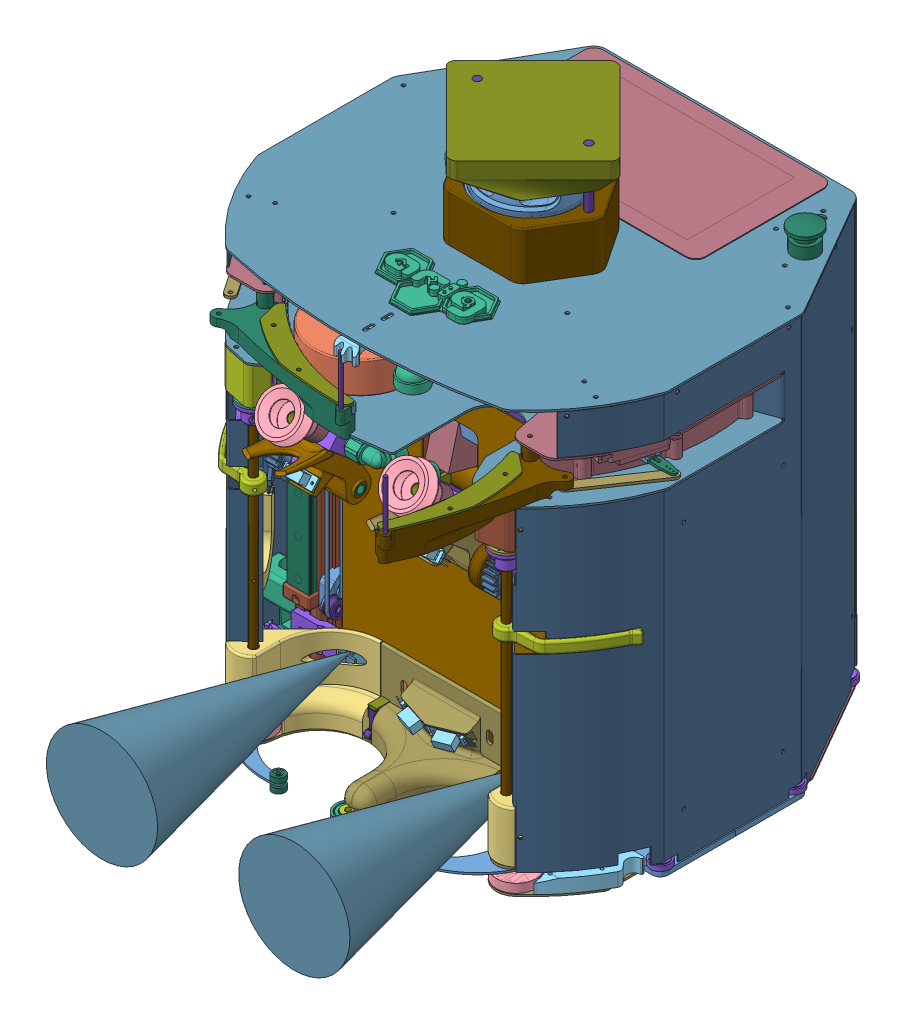
SolidWorks assembly 2019_Gros_robot, configuration Défaut. Lengths in mm. (continued)
Components (placement in the parent): (continued)
- 20181005-1508-1: 20181005-1508 [Défaut] at (-50 277.5 -86.6025) x (0 0 1) z (-1 0 0) size (212.1 303.52 220.42)
  - 20181005-1449-1: 20181005-1449 [Défaut] at (-40 0 0) size (80 80 0) (hidden)
  - 20181005-1520-1: 20181005-1520 [Défaut] at (40 -35 0) x (-0.992278 0.124035 0) z (0 0 -1) size (48.31 18.76 50.57)
  - 20181005-1525-1: 20181005-1525 [Défaut] at (30 -50 0) x (-0.986394 0.164399 0) z (0 0 -1) size (38.41 16.66 50.83)
  - 20181005-1532-1: 20181005-1532 [Défaut] at origin size (84 50 84)
  - Rotule Rose-1: Rotule Rose [aligné] at (33.0169 -69.1373 7) x (0.894203 -0.447662 0) z (-0.447662 -0.894203 0) size (18 6.89 7.5)
    - Rotule Rose piece01-1: Rotule Rose piece01 [Défaut] at origin size (5.4 6 5.4)
    - Rotule Rose piece02-1: Rotule Rose piece02 [Défaut] x (-1 0 0) z (0 0 -1) size (18 5.77 7.5)
  - Rotule noire-2: Rotule noire [Aligné] at (3.5082 -54.3644 7) x (0.894203 -0.447662 0) z (-0.447662 -0.894203 0) size (19 15.5 6.5)
    - Rotule noire piece01-1: Rotule noire piece01 [Défaut] at origin size (6.35 14.5 5.5)
    - Rotule noire piece02-1: Rotule noire piece02 [Défaut] at origin size (19 6 6.5)
  - Rondelle-M3-1: Rondelle-M3 [Défaut] at (40 -35 25) x (0.373687 0.927555 0) z (0 0 1) size (8 8 0.8)
  - EcrouFrein_H-M3-1: EcrouFrein_H-M3 [Défaut] at (40 -35 25.8) x (0.960386 -0.278675 0) z (0 0 1) size (6.35 5.5 4)
  - Rondelle-M3-3: Rondelle-M3 [Défaut] at (30 -50 20.2) x (0.958956 -0.283556 0) z (0 0 1) size (8 8 0.8)
  - Rondelle-M3-4: Rondelle-M3 [Défaut] at (30 -50 25) size (8 8 0.8)
  - EcrouFrein_H-M3-2: EcrouFrein_H-M3 [Défaut] at (30 -50 25.8) x (0.755806 -0.654795 0) z (0 0 1) size (6.35 5.5 4)
  - Rondelle-M3-5: Rondelle-M3 [Défaut] at (40 -35 20.2) x (0.958956 -0.283556 0) z (0 0 1) size (8 8 0.8)
  - Rondelle-M3-6: Rondelle-M3 [Défaut] at (0 -45 22.5) size (8 8 0.8)
  - Rondelle-M3-7: Rondelle-M3 [Défaut] at (0 -45 17.7) x (0.958956 -0.283556 0) z (0 0 1) size (8 8 0.8)
  - Rondelle-M3-8: Rondelle-M3 [Défaut] at (0 -30 22.5) size (8 8 0.8)
  - Rondelle-M3-9: Rondelle-M3 [Défaut] at (0 -30 17.7) x (0.958956 -0.283556 0) z (0 0 1) size (8 8 0.8)
  - EcrouFrein_H-M3-3: EcrouFrein_H-M3 [Défaut] at (0 -45 23.3) x (0.755806 -0.654795 0) z (0 0 1) size (6.35 5.5 4)
  - EcrouFrein_H-M3-4: EcrouFrein_H-M3 [Défaut] at (0 -30 23.3) x (0.755806 -0.654795 0) z (0 0 1) size (6.35 5.5 4)
  - EcrouFrein_H-M3-5: EcrouFrein_H-M3 [Défaut] at (0 -45 -23.3) x (-0.328469 -0.944515 0) z (0 0 -1) size (6.35 5.5 4)
  - Rondelle-M3-10: Rondelle-M3 [Défaut] at (0 -45 -23.3) size (8 8 0.8)
  - Rondelle-M3-11: Rondelle-M3 [Défaut] at (0 -45 -18.5) size (8 8 0.8)
  - Rondelle-M3-12: Rondelle-M3 [Défaut] at (0 -30 -18.5) size (8 8 0.8)
  - Rondelle-M3-13: Rondelle-M3 [Défaut] at (0 -30 -23.3) size (8 8 0.8)
  - EcrouFrein_H-M3-6: EcrouFrein_H-M3 [Défaut] at (0 -30 -23.3) x (-0.328469 -0.944515 0) z (0 0 -1) size (6.35 5.5 4)
  - Rondelle-M3-14: Rondelle-M3 [Défaut] at (40 -35 -25.8) size (8 8 0.8)
  - EcrouFrein_H-M3-7: EcrouFrein_H-M3 [Défaut] at (40 -35 -25.8) x (-0.328469 -0.944515 0) z (0 0 -1) size (6.35 5.5 4)
  - Rondelle-M3-15: Rondelle-M3 [Défaut] at (40 -35 -21) size (8 8 0.8)
  - Rondelle-M3-16: Rondelle-M3 [Défaut] at (30 -50 -21) size (8 8 0.8)
  - Rondelle-M3-17: Rondelle-M3 [Défaut] at (30 -50 -25.8) size (8 8 0.8)
  - EcrouFrein_H-M3-8: EcrouFrein_H-M3 [Défaut] at (30 -50 -25.8) x (-0.328469 -0.944515 0) z (0 0 -1) size (6.35 5.5 4)
  - Palet-1: Palet [Redium] at (0 12.7 0) size (76.2 25.4 76.2)
  - 20181005-2259-1: 20181005-2259 [Défaut] at (-69.4 -270.5 0) size (84 270.5 220.42) (hidden)
  - Palet-2: Palet [Redium] at (-54.2246 -232.142 0) x (0.022904 0.999738 0) z (0 0 1) size (76.2 25.4 76.2)
  - Palet-3: Palet [Redium] at (-52.4793 -155.962 0) x (-0.022904 -0.999738 0) z (0 0 -1) size (76.2 25.4 76.2)
  - Palet-4: Palet [Redium] at (-57 -79.3665 0) x (0.005796 0.999983 0) z (0 0 1) size (76.2 25.4 76.2)
  - 20181006-0057-1: 20181006-0057 [Défaut] at (40 -35 0) size (109.6 110.42 46)
  - 20181006-0127-1: 20181006-0127 [Défaut] at (5.6 -53.5947 -48) size (47 24.09 104)
  - Igus_TK_04_09_Rail_L50-1: Igus_TK_04_09_Rail_L50 [Défaut] at (-10.4 -270.5 0) x (0 0 -1) z (0 1 0) size (9.6 50 6.3)
  - Igus_TK_04_09_coulisseau-1: Igus_TK_04_09_coulisseau [Défaut] at (-78.9 -270.5 0) x (0 0 -1) z (0 1 0) size (20 29 8.3)
  - 20181006-1513-1: 20181006-1513 [Défaut] at (-20.9 -260.5 0) x (0 0 1) z (-1 0 0) size (55 3 30) (hidden)
  - 20181006-1518-1: 20181006-1518 [Défaut] at (-5.9 -265.85 -24) x (0 0 1) z (-1 0 0) size (7.5 7.5 65) (hidden)
  - 20181006-1518-2: 20181006-1518 [Défaut] at (-5.9 -265.85 24) x (0 0 -1) z (-1 0 0) size (7.5 7.5 65) (hidden)
  - Servo_HS-485-HB-1: Servo_HS-485-HB [Default] at (55 -70 -42.29) x (-1 0 0) z (0 0 1) size (19.81 54.15 42.74)
  - Access_HS-485_BrasReglablePartieA-1: Access_HS-485_BrasReglablePartieA [Défaut] at (55 -70 0.45) x (0.039215 0.999231 0) z (0.999231 -0.039215 0) size (10 6 10)
  - Access_HS-485_BrasReglablePartieB-1: Access_HS-485_BrasReglablePartieB [Défaut] at (55.9992 -70.0392 1.45) x (0.039215 0.999231 0) z (0.999231 -0.039215 0) size (7.5 2 30.5)
  - Servo_HS-485-HB-2: Servo_HS-485-HB [Default] at (-17.4 -237.5 -49.74) x (-1 0 0) z (0 0 1) size (19.81 54.15 42.74)
  - microswitchGaletAss-1: microswitchGaletAss [Défaut] at (50 -23 -29.5) x (0 1 0) z (0 0 1) size (21.06 21.1 7)
    - microswitchGalet02-1: microswitchGalet02 [Défaut] at origin size (20 15 7)
    - microswitchGalet01-1: microswitchGalet01 [Défaut] at (1.7099 12.1145 0) x (0.996636 -0.081957 0) z (0 0 1) size (19 9 6)
  - Access_HS-645_BrasRondPetitModele-1: Access_HS-645_BrasRondPetitModele [Défaut] at (-17.4 -237.5 -10) x (0.340211 -0.940349 0) z (-0.940349 -0.340211 0) size (24 5 24)
  - Servo_HS-485-HB-3: Servo_HS-485-HB [Default] at (-17.4 -237.5 -50.26) x (1 0 0) z (0 0 -1) size (19.81 54.15 42.74)
  - Access_HS-645_BrasRondPetitModele-2: Access_HS-645_BrasRondPetitModele [Défaut] at (-17.4 -237.5 -90) x (0.232733 0.972541 0) z (-0.972541 0.232733 0) size (24 5 24)
  - 20190325-2254-1: 20190325-2254 [Défaut] at (-5.9 -256.5 0) x (0 0 1) z (-1 0 0) size (56 23 30)
  - 20190325-2336-1: 20190325-2336 [Défaut] at (-17.4 -237.5 -5.5) x (-0.001924 -0.999998 0) z (0 0 1) size (24 31 4)
  - 20190325-2347-1: 20190325-2347 [Défaut] at (-32.4 -237.4711 -1.5) x (0.865384 -0.50111 0) z (0 0 1) size (33.5 7.5 1.5)
  - 20190326-0009-1: 20190326-0009 [Défaut] at (-5.9 -265.5 25) x (0 0 1) z (-1 0 0) size (8 8 65)
  - 20190326-0009-2: 20190326-0009 [Défaut] at (-5.9 -265.5 -25) x (0 0 1) z (-1 0 0) size (8 8 65)
  - 20190327-2029-1: 20190327-2029 [Défaut] at (-69.4011 -269.4991 -50) size (23.86 187.02 200)
  - 20190327-2138-1: 20190327-2138 [Défaut] at (-17.4 -227.5 -50) size (40 70 54)
  - microswitchGaletAss-2: microswitchGaletAss [Défaut] at (-59.4 -233 47.5) x (0 -1 0) z (0 0 -1) size (21.06 21.1 7)
    - microswitchGalet02-1: microswitchGalet02 [Défaut] at origin size (20 15 7)
    - microswitchGalet01-1: microswitchGalet01 [Défaut] at (1.7099 12.1145 0) x (0.996636 -0.081957 0) z (0 0 1) size (19 9 6)
  - 20190328-2330-1: 20190328-2330 [Défaut] at (-69.4 -270.5 0) size (84 269 20.21)
  - 20190328-2332-1: 20190328-2332 [Défaut] at (-69.4 -270.5 0) size (84 270.5 20)
  - Symétrie20190328-2330-2: Symétrie20190328-2330 [Défaut] at (-69.4 -270.5 -100) size (84 269 20.21)
  - Symétrie20181006-0057-2: Symétrie20181006-0057 [Défaut] at (40 -35 -100) size (109.6 110.42 46)
  - 20181005-1532-2: 20181005-1532 [Défaut] at (0 0 -100) size (84 50 84)
  - Servo_HS-485-HB-4: Servo_HS-485-HB [Default] at (55 -49.85 -57.71) x (-1 0 0) z (0 0 -1) size (19.81 54.15 42.74)
  - Access_HS-485_BrasReglablePartieA-2: Access_HS-485_BrasReglablePartieA [Défaut] at (55 -70 -100.45) x (0.039215 0.999231 0) z (-0.999231 0.039215 0) size (10 6 10)
  - Access_HS-485_BrasReglablePartieB-2: Access_HS-485_BrasReglablePartieB [Défaut] at (55.9992 -70.0392 -101.45) x (-0.039215 -0.999231 0) z (0.999231 -0.039215 0) size (7.5 2 30.5)
  - Rotule Rose-2: Rotule Rose [aligné] at (33.0169 -69.1373 -107) x (0.894203 -0.447662 0) z (0.447662 0.894203 0) size (18 6.89 7.5)
    - Rotule Rose piece01-1: Rotule Rose piece01 [Défaut] at origin size (5.4 6 5.4)
    - Rotule Rose piece02-1: Rotule Rose piece02 [Défaut] x (-1 0 0) z (0 0 -1) size (18 5.77 7.5)
  - Rotule noire-3: Rotule noire [Aligné] at (3.5082 -54.3644 -107) x (0.894203 -0.447662 0) z (0.447662 0.894203 0) size (19 15.5 6.5)
    - Rotule noire piece01-1: Rotule noire piece01 [Défaut] at origin size (6.35 14.5 5.5)
    - Rotule noire piece02-1: Rotule noire piece02 [Défaut] at origin size (19 6 6.5)
  - Symétrie20181006-0127-2: Symétrie20181006-0127 [Défaut] at (5.6 -53.5947 -52) size (47 24.09 104)
  - Igus_TK_04_09_Rail_L50-2: Igus_TK_04_09_Rail_L50 [Défaut] at (-10.4 -270.5 -100) x (0 0 -1) z (0 1 0) size (9.6 50 6.3)
  - Igus_TK_04_09_coulisseau-2: Igus_TK_04_09_coulisseau [Défaut] at (-78.9 -258.8 -100) x (0 0 1) z (0 -1 0) size (20 29 8.3)
  - Symétrie20190325-2254-2: Symétrie20190325-2254 [Défaut] at (-5.9 -256.5 -100) x (0 0 -1) z (1 0 0) size (56 23 30)
  - 20190326-0009-3: 20190326-0009 [Défaut] at (-5.9 -265.5 -125) x (0 0 1) z (-1 0 0) size (8 8 65)
  - 20190326-0009-4: 20190326-0009 [Défaut] at (-5.9 -265.5 -75) x (0 0 1) z (-1 0 0) size (8 8 65)
  - 20190325-2347-2: 20190325-2347 [Défaut] at (-32.4 -237.4711 -100) x (0.865384 -0.50111 0) z (0 0 1) size (33.5 7.5 1.5)
  - 20190325-2336-2: 20190325-2336 [Défaut] at (-17.4 -237.5 -94.5) x (0.001924 0.999998 0) z (0 0 -1) size (24 31 4)
  - EcrouFrein_H-M3-9: EcrouFrein_H-M3 [Défaut] at (40 -35 -74.2) x (0.328469 0.944515 0) z (0 0 1) size (6.35 5.5 4)
  - EcrouFrein_H-M3-10: EcrouFrein_H-M3 [Défaut] at (0 -30 -76.7) x (0.328469 0.944515 0) z (0 0 1) size (6.35 5.5 4)
  - Rondelle-M3-18: Rondelle-M3 [Défaut] at (0 -30 -77.5) size (8 8 0.8)
  - Rondelle-M3-19: Rondelle-M3 [Défaut] at (0 -45 -77.5) size (8 8 0.8)
  - EcrouFrein_H-M3-11: EcrouFrein_H-M3 [Défaut] at (0 -45 -76.7) x (0.328469 0.944515 0) z (0 0 1) size (6.35 5.5 4)
  - Rondelle-M3-20: Rondelle-M3 [Défaut] at (30 -50 -75) size (8 8 0.8)
  - EcrouFrein_H-M3-12: EcrouFrein_H-M3 [Défaut] at (30 -50 -74.2) x (0.328469 0.944515 0) z (0 0 1) size (6.35 5.5 4)
  - Rondelle-M3-21: Rondelle-M3 [Défaut] at (30 -50 -79.8) size (8 8 0.8)
  - 20181005-1525-2: 20181005-1525 [Défaut] at (30 -50 -100) x (-0.986394 0.164399 0) z (0 0 -1) size (38.41 16.66 50.83)
  - Rondelle-M3-22: Rondelle-M3 [Défaut] at (40 -35 -75) size (8 8 0.8)
  - Rondelle-M3-23: Rondelle-M3 [Défaut] at (40 -35 -79.8) size (8 8 0.8)
  - 20181005-1520-2: 20181005-1520 [Défaut] at (40 -35 -100) x (-0.992278 0.124035 0) z (0 0 -1) size (48.31 18.76 50.57)
  - Rondelle-M3-24: Rondelle-M3 [Défaut] at (0 -30 -82.3) size (8 8 0.8)
  - Rondelle-M3-25: Rondelle-M3 [Défaut] at (0 -45 -82.3) size (8 8 0.8)
  - Rondelle-M3-26: Rondelle-M3 [Défaut] at (0 -45 -118.5) x (0.958956 -0.283556 0) z (0 0 1) size (8 8 0.8)
  - Rondelle-M3-27: Rondelle-M3 [Défaut] at (0 -45 -123.3) size (8 8 0.8)
  - EcrouFrein_H-M3-13: EcrouFrein_H-M3 [Défaut] at (0 -45 -123.3) x (-0.755806 0.654795 0) z (0 0 -1) size (6.35 5.5 4)
  - Rondelle-M3-28: Rondelle-M3 [Défaut] at (0 -30 -123.3) size (8 8 0.8)
  - EcrouFrein_H-M3-14: EcrouFrein_H-M3 [Défaut] at (0 -30 -123.3) x (-0.755806 0.654795 0) z (0 0 -1) size (6.35 5.5 4)
  - Rondelle-M3-29: Rondelle-M3 [Défaut] at (30 -50 -121) x (0.958956 -0.283556 0) z (0 0 1) size (8 8 0.8)
  - Rondelle-M3-30: Rondelle-M3 [Défaut] at (30 -50 -125.8) size (8 8 0.8)
  - EcrouFrein_H-M3-15: EcrouFrein_H-M3 [Défaut] at (30 -50 -125.8) x (-0.755806 0.654795 0) z (0 0 -1) size (6.35 5.5 4)
  - Rondelle-M3-31: Rondelle-M3 [Défaut] at (40 -35 -121) x (0.958956 -0.283556 0) z (0 0 1) size (8 8 0.8)
  - Rondelle-M3-32: Rondelle-M3 [Défaut] at (40 -35 -125.8) x (0.373687 0.927555 0) z (0 0 1) size (8 8 0.8)
  - EcrouFrein_H-M3-16: EcrouFrein_H-M3 [Défaut] at (40 -35 -125.8) x (-0.960386 0.278675 0) z (0 0 -1) size (6.35 5.5 4)
  - Rondelle-M3-33: Rondelle-M3 [Défaut] at (0 -30 -118.5) x (0.958956 -0.283556 0) z (0 0 1) size (8 8 0.8)
  - microswitchGaletAss-3: microswitchGaletAss [Défaut] at (50 -23 -70.5) x (0 1 0) z (0 0 1) size (21.06 21.1 7)
    - microswitchGalet02-1: microswitchGalet02 [Défaut] at origin size (20 15 7)
    - microswitchGalet01-1: microswitchGalet01 [Défaut] at (1.7099 12.1145 0) x (0.996636 -0.081957 0) z (0 0 1) size (19 9 6)
  - microswitchGaletAss-4: microswitchGaletAss [Défaut] at (-59.4 -233 -147.5) x (0 -1 0) z (0 0 -1) size (21.06 21.1 7)
    - microswitchGalet02-1: microswitchGalet02 [Défaut] at origin size (20 15 7)
    - microswitchGalet01-1: microswitchGalet01 [Défaut] at (1.7099 12.1145 0) x (0.996636 -0.081957 0) z (0 0 1) size (19 9 6)
- 20181006-0254-1: 20181006-0254 [Défaut] at (0 343.5 -160.0025) size (213 210 4)
- Palet-1: Palet [Redium] at (-50 12.7 119.5978) size (76.2 25.4 76.2) (hidden)
- Raspberry pi3 Screen assembly-1: Raspberry pi3 Screen assembly [Défaut] at (-26.2349 344.907 -108.8519) x (0.999654 0 -0.026321) z (0 1 0) size (195.4 115.39 39.45)
- Carte alimentation convertisseur-1: Carte alimentation convertisseur [Défaut] at (195.1731 449.8125 151.3603) size (102.6 19 94) (hidden)
- Interf Raspi-1: Interf Raspi [Défaut] at (205.7046 396.6201 128.2669) size (80.1 34 58.6) (hidden)
- Capteurs Analogique-1: Capteurs Analogique [Défaut] at (234.5762 364.7789 172.5689) size (27.2 19 38.1) (hidden)
- Capteurs Numerique-1: Capteurs Numerique [Défaut] at (209.8881 326.819 165.4886) size (43.6 19 47.8) (hidden)
- SD21-1: SD21 [Défaut] at (239.2416 462.0315 160.3108) size (50 30 85) (hidden)
- Carte codeur v2-1: Carte codeur v2 [Défaut] at (181.4763 130.2292 111.0518) size (54.1 39 54.4) (hidden)
- Carte codeur v1-1: Carte codeur v1 [Défaut] at (219.0947 57.0207 83.9025) size (42.8 24 53.9) (hidden)
- pompe air 12v SFE-2: pompe air 12v SFE [Défaut] at (20.3606 32 -38) size (38 60 92)
- BillePorteuse2019-1: BillePorteuse2019 [Défaut] at (105.917 0 116.9526) x (0.630519 0 -0.776174) z (0.776174 0 0.630519) size (16 10 16)
- microswitchGaletAss-1: microswitchGaletAss [Défaut] at (50 29 66) x (0 -1 0) z (-1 0 0) size (21.06 21.1 7)
  - microswitchGalet02-1: microswitchGalet02 [Défaut] at origin size (20 15 7)
  - microswitchGalet01-1: microswitchGalet01 [Défaut] at (1.7099 12.1145 0) x (0.996636 -0.081957 0) z (0 0 1) size (19 9 6)
- Roulement_d3xd10xe4-1: Roulement_d3xd10xe4 [Défaut] at (45.0929 15.95 157.5553) x (0 1 0) z (-0.541709 0 -0.840566) size (4 10 10)
- roulement-1: roulement [Défaut] at (0 11.5 145.4518) x (0 -1 0) z (0.861176 0 0.508306) size (7 22 22)
- Servo_HS-485-HB-1: Servo_HS-485-HB [Default] at (148.2228 335.79 52.8032) x (-0.95652 0 -0.291667) z (0 -1 0) size (19.81 54.15 42.74)
- Access_HS-485_BrasReglablePartieB-1: Access_HS-485_BrasReglablePartieB [Défaut] at (147.2257 292.05 52.7272) x (0.076016 0 -0.997107) z (-0.997107 0 -0.076016) size (7.5 2 30.5)
- Access_HS-485_BrasReglablePartieA-1: Access_HS-485_BrasReglablePartieA [Défaut] at (148.2228 293.05 52.8032) x (0.076016 0 -0.997107) z (-0.997107 0 -0.076016) size (10 6 10)
- 20190123-2208-1: 20190123-2208 [Défaut] at (0 8.1 145.4518) size (11.85 7.9 11.85)
- Electrovanne12VDC-1: Electrovanne12VDC [Défaut] at (47 164.0788 27.5) x (0 -1 0) z (0 0 1) size (36.5 64 22)
- CapteurVide_CKD_PPE-V01A-H6-B-1: CapteurVide_CKD_PPE-V01A-H6-B [Défaut] at (90 114.0788 27.5) x (0 -1 0) z (0 0 1) size (37 43 15)
- CarteVentillo-1: CarteVentillo [Défaut] at (248.165 281.582 64.2045) size (50 15 43) (hidden)
- 20190208-2148-1: 20190208-2148 [Défaut] at (102 60.4 120.9526) x (0.640285 0 0.768138) z (0 1 0) size (6 6 175)
- 20190208-2207-1: 20190208-2207 [Défaut] at (102.5 18.75 117.5) x (-0.820101 0 0.572218) z (-0.572218 0 -0.820101) size (86 1.5 31.58)
- Roulement_d3xd10xe4-2: Roulement_d3xd10xe4 [Défaut] at (45.0929 23.05 157.5553) x (0 1 0) z (-0.268999 0 0.963141) size (4 10 10)
- Servo_HS-85-BB-1: Servo_HS-85-BB [Défaut] at (102.5 25.85 117.5) x (1 0 0) z (0 -1 0) size (13 41.3 34.1)
- 20190212-2200-1: 20190212-2200 [Défaut] at (-50 7 120) size (239.52 60.05 68.05)
- 20190214-0012-1: 20190214-0012 [Défaut] at (105.917 7.7 116.9526) x (0.866025 0 -0.5) z (0.5 0 0.866025) size (32 10 32)
- Access_HS-645_BrasRondPetitModele-1: Access_HS-645_BrasRondPetitModele [Défaut] at (102.5 24.75 117.5) x (-0.643539 0 0.765413) z (0.765413 0 0.643539) size (24 5 24)
- 20190208-2207-2: 20190208-2207 [Défaut] at (102.5 18.75 117.5) x (0.794361 0 -0.607446) z (0.607446 0 0.794361) size (86 1.5 31.58) (hidden)
- 20170416-2304-1: 20170416-2304 [Défaut] at (12.2889 46.5676 67.2799) x (0.965926 0.109382 -0.23457) z (0.258819 -0.408218 0.875426) size (30.6 16 70.4)
  - SupportCapteurPololu-1: SupportCapteurPololu [Défaut] at origin size (30 16 12.5) (hidden)
  - pololu gp2y0d805-1: pololu gp2y0d805 [Défaut] at (-14.5 -4.5 10.8) size (30.1 9 11.8)
  - faisceau pololu gp2y0d-1: faisceau pololu gp2y0d [5cm] at (-3.9 0 20.4) size (2 2 50) (hidden)
- 20190219-0006-1: 20190219-0006 [Défaut] at (0 7 0) size (30.83 11 59.43)
- Roulement_d3xd10xe4-3: Roulement_d3xd10xe4 [Défaut] at (158.1053 15.95 74.9788) x (0 1 0) z (-0.541709 0 -0.840566) size (4 10 10) (hidden)
- 20190219-0101-1: 20190219-0101 [Défaut] at (130 51.0678 50) x (0 0 -1) z (1 0 0) size (22 20 34.5)
- 20190219-0101-2: 20190219-0101 [Défaut] at (130 51.0678 -50) x (0 0 1) z (1 0 0) size (22 20 34.5)
- 20190220-2148-1: 20190220-2148 [Défaut] at (102 181.4 120.9526) x (0.406737 0 -0.913545) z (0.913545 0 0.406737) size (78.13 10.25 45.74)
- Servo_HS-85-BB-2: Servo_HS-85-BB [Défaut] at (102 246 120.9526) x (0.5 0 0.866025) z (0 -1 0) size (13 41.3 34.1)
- Access_HS-645_BrasRondPetitModele-2: Access_HS-645_BrasRondPetitModele [Défaut] at (102 244.9 120.9526) x (-0.940804 0 0.338952) z (0.338952 0 0.940804) size (24 5 24)
- 20190221-0033-1: 20190221-0033 [Défaut] at (102 240.4 120.9526) x (-0.640285 0 -0.768138) z (-0.768138 0 0.640285) size (24 15 24)
- 20190221-0152-1: 20190221-0152 [Défaut] at (0 312.2 0) x (-1 0 0) z (0 0 1) size (65.17 50 53.91)
- Carter2019-1: Carter2019 [Défaut] at (0 7 0) size (63.71 336 283.98)
- 20190223-1730-1: 20190223-1730 [Défaut] at (-0.1299 256 0.1276) size (48.99 30 36.97)
- 20170416-2304-2: 20170416-2304 [Défaut] at (-12.2889 46.5676 67.2799) x (-0.965926 0.109382 -0.23457) z (-0.258819 -0.408218 0.875426) size (30.6 16 70.4)
  - SupportCapteurPololu-1: SupportCapteurPololu [Défaut] at origin size (30 16 12.5) (hidden)
  - pololu gp2y0d805-1: pololu gp2y0d805 [Défaut] at (-14.5 -4.5 10.8) size (30.1 9 11.8)
  - faisceau pololu gp2y0d-1: faisceau pololu gp2y0d [5cm] at (-3.9 0 20.4) size (2 2 50) (hidden)
- 20190225-2214-1: 20190225-2214 [Défaut] at (134.7726 288.5 106.5984) x (0.561691 0 -0.827347) z (0.827347 0 0.561691) size (71 2 8)
- Robot2019_plaque elec-1: Robot2019_plaque elec [Défaut] at (0 309.5 0) size (330 1.5 265.02)
- Robot2019_plaque superieure-2: Robot2019_plaque superieure [Défaut] at (0 343.5 0) size (330 1.5 305)
- 20161105-0900-1: 20161105-0900 [Défaut] at (0 345 0) size (105 35.5 75)
- 20190313-2117-1: 20190313-2117 [Défaut] at (0 430 -2.5) x (-1 0 0) z (0 0 1) size (135.87 27.01 134.45)
- 20161106-1538-1: 20161106-1538 [Défaut] at (-45 350 -2.5) size (6 80 6)
- 20161106-1538-2: 20161106-1538 [Défaut] at (45 350 -2.5) size (6 80 6)
- 20170416-2304-3: 20170416-2304 [Défaut] at (-120 226 -15) x (0 0 -1) z (0 1 0) size (30.6 16 70.4)
  - SupportCapteurPololu-1: SupportCapteurPololu [Défaut] at origin size (30 16 12.5) (hidden)
  - pololu gp2y0d805-1: pololu gp2y0d805 [Défaut] at (-14.5 -4.5 10.8) size (30.1 9 11.8)
  - faisceau pololu gp2y0d-1: faisceau pololu gp2y0d [5cm] at (-3.9 0 20.4) size (2 2 50) (hidden)
- Adafruit_TCS34725-1: Adafruit_TCS34725 [Défaut] at (-106.6 273 31) x (0 0 -1) z (0 1 0) size (20.5 20.4 5)
- 20190227-2336-1: 20190227-2336 [Défaut] at (-120 256.5 40) x (-1 0 0) z (0 0 -1) size (17 25 31.5)
- 20190228-0009-1: 20190228-0009 [Défaut] at (0 165.5788 39.25) x (0 0 -1) z (-1 0 0) size (19.5 19.5 255)
- Robot2015_supportServo02-1: Robot2015_supportServo02 [Défaut] at (-34 217.5 -3.6025) x (0 0 -1) z (1 0 0) size (38 65 1.5)
- 20190301-2106-1: 20190301-2106 [Défaut] at (47.184 337.04 -102.825) x (-1 0 0) z (0 0 -1) size (55 8.5 82)
- 20190301-2139-1: 20190301-2139 [Défaut] at (0 343.5 0) size (18.21 12.25 42)
- LogoARIG2-1: LogoARIG2 [Défaut] at (-42.5 345 104) x (1 0 0) z (0 1 0) size (88.08 45.8 6.03)
- GP2D-2: GP2D [Défaut] at (75 287.5 -145) x (-1 0 0) z (0 0 1) size (44.5 15.5 19)
- 20190301-2106-2: 20190301-2106 [Défaut] at (-63.016 337.04 -102.825) size (55 8.5 82)
- LogoARIG2-2: LogoARIG2 [Défaut] at (42.5 244.5 -160.0025) x (-1 0 0) z (0 0 -1) size (88.08 45.8 6.03)
- 20190308-1510-1: 20190308-1510 [Défaut] at (0 336.5 0) size (33.55 41 203.81)
- interrupteur principal-1: interrupteur principal [Défaut] at (145.1715 323 -71.7856) x (0.5 0 0.866025) z (0 1 0) size (32 33.35 25)
- 20190308-2149-1: 20190308-2149 [Défaut] at (0 343.5 0) x (-1 0 0) z (0 0 1) size (43.23 7 234.12)
- 20190309-0049-1: 20190309-0049 [Défaut] at (0 311 43) size (178.08 32 17)
- 20190309-0127_Corniere_15.5x27.5x1.5-1: 20190309-0127_Corniere_15.5x27.5x1.5 [Défaut] at (-130 276 -59) x (-1 0 0) z (0 0 1) size (27.5 15.5 118)
- Ventilo-2: Ventilo [Défaut] at (75 318.5 -156.0025) size (40 40 11.91)
- TelemetreTOF_RB-Mce-01-1: TelemetreTOF_RB-Mce-01 [Défaut] at (-74.5065 272.4886 -143) x (0 0 1) z (0.139173 -0.990268 0) size (89.68 89.68 210)
- Ventilo-3: Ventilo [Défaut] at (0 318.5 -156.0025) size (40 40 11.91)
- Ventilo-4: Ventilo [Défaut] at (-75 318.5 -156.0025) size (40 40 11.91)
- 20190314-1109-1: 20190314-1109 [Défaut] at (-74.5065 272.4886 -143) x (0 0 1) z (-0.990268 -0.139173 0) size (25 4.81 20)
- 20181006-0255-1: 20181006-0255 [Défaut] at (0 133.2 -160.0025) size (213 80 4)
- Palet-2: Palet [Redium] at (51.9 38.1 -143.8025) x (0 1 0) z (-1 0 0) size (76.2 25.4 76.2) (hidden)
- TelemetreTOF_RB-Mce-01-2: TelemetreTOF_RB-Mce-01 [Défaut] at (77.5 42 64.5) size (89.68 89.68 210)
- 20190331-1440-1: 20190331-1440 [Défaut] at (77.5 42 64.5) x (1 0 0) z (0 1 0) size (65.5 6.5 20)
- 20190331-1545-1: 20190331-1545 [Défaut] at (0 383.5 -2.5) x (-1 0 0) z (0 0 1) size (110 38.3 83)
- 20190331-1640-1: 20190331-1640 [Défaut] at (0 257 22.5) size (90 54 43)
- 20190309-0128-1: 20190309-0128 [Défaut] at (-130 276 -59) x (-1 0 0) z (0 0 1) size (27.02 16 119.7)
- SupportCapteurPololuSpecial2019-1: SupportCapteurPololuSpecial2019 [Défaut] at (-120 226 -15) x (0 0 -1) z (0 1 0) size (41.3 16 24)
- Robot2015_BaseRoulante_piece15-1: Robot2015_BaseRoulante_piece15 [Défaut] at (-95 79.5 -60) x (0 0 -1) z (1 0 0) size (40 40 190)
- Symétrie20190219-0006-2: Symétrie20190219-0006 [Défaut] at (0 7 0) x (-1 0 0) z (0 0 -1) size (30.83 11 59.43)
- microswitchGaletAss-2: microswitchGaletAss [Défaut] at (-50 29 66) x (0 -1 0) z (-1 0 0) size (21.06 21.1 7)
  - microswitchGalet02-1: microswitchGalet02 [Défaut] at origin size (20 15 7)
  - microswitchGalet01-1: microswitchGalet01 [Défaut] at (1.7099 12.1145 0) x (0.996636 -0.081957 0) z (0 0 1) size (19 9 6)
- 20190208-2207-3: 20190208-2207 [Défaut] at (-102.5 20.25 117.5) x (0.820101 0 0.572218) z (0.572218 0 -0.820101) size (86 1.5 31.58)
- Roulement_d3xd10xe4-4: Roulement_d3xd10xe4 [Défaut] at (-45.0929 23.05 157.5553) x (0 1 0) z (-0.268999 0 -0.963141) size (4 10 10)
- Roulement_d3xd10xe4-5: Roulement_d3xd10xe4 [Défaut] at (-45.0929 15.95 157.5553) x (0 1 0) z (-0.541709 0 0.840566) size (4 10 10)
- Access_HS-645_BrasRondPetitModele-3: Access_HS-645_BrasRondPetitModele [Défaut] at (-102.5 19.75 117.5) x (0.643539 0 0.765413) z (-0.765413 0 0.643539) size (24 5 24)
- 20190214-0012-2: 20190214-0012 [Défaut] at (-105.917 7.7 116.9526) x (0.866025 0 0.5) z (-0.5 0 0.866025) size (32 10 32)
- BillePorteuse2019-2: BillePorteuse2019 [Défaut] at (-105.917 0 116.9526) x (-0.630519 0 -0.776174) z (0.776174 0 -0.630519) size (16 10 16)
- 20190208-2148-2: 20190208-2148 [Défaut] at (-102 235.4 120.9526) x (-0.640285 0 0.768138) z (0 -1 0) size (6 6 175)
- 20190220-2148-2: 20190220-2148 [Défaut] at (-102 181.4 120.9526) x (-0.406737 0 -0.913545) z (-0.913545 0 0.406737) size (78.13 10.25 45.74)
- 20190221-0033-2: 20190221-0033 [Défaut] at (-102 240.4 120.9526) x (-0.640285 0 0.768138) z (0.768138 0 0.640285) size (24 15 24)
- SymétrieAccess_HS-645_BrasRondPetitModele-4: SymétrieAccess_HS-645_BrasRondPetitModele [Défaut] at (-102 244.9 120.9526) x (0.940804 0 0.338952) z (0.338952 0 -0.940804) size (24 5 24)
- Symétrie20190223-1730-2: Symétrie20190223-1730 [Défaut] at (0.1299 256 0.1276) x (-1 0 0) z (0 0 -1) size (48.99 30 36.97)
- Servo_HS-85-BB-3: Servo_HS-85-BB [Défaut] at (-102.5 25.85 101.5) x (-1 0 0) z (0 -1 0) size (13 41.3 34.1)
- Symétrie20190331-1440-2: Symétrie20190331-1440 [Défaut] at (-77.5 42 64.5) x (-1 0 0) z (0 -1 0) size (65.5 6.5 20)
- Servo_HS-85-BB-4: Servo_HS-85-BB [Défaut] at (-102 246 120.9526) x (0.5 0 -0.866025) z (0 -1 0) size (13 41.3 34.1)
- Servo_HS-485-HB-2: Servo_HS-485-HB [Default] at (-148.2228 335.79 52.8032) x (-0.95652 0 0.291667) z (0 -1 0) size (19.81 54.15 42.74)
- Access_HS-485_BrasReglablePartieA-2: Access_HS-485_BrasReglablePartieA [Défaut] at (-148.2228 293.05 52.8032) x (-0.076016 0 -0.997107) z (-0.997107 0 0.076016) size (10 6 10)
- Access_HS-485_BrasReglablePartieB-2: Access_HS-485_BrasReglablePartieB [Défaut] at (-147.2257 292.05 52.7272) x (0.076016 0 0.997107) z (0.997107 0 -0.076016) size (7.5 2 30.5)
- 20190225-2214-2: 20190225-2214 [Défaut] at (-134.7726 288.5 106.5984) x (-0.561691 0 -0.827347) z (0.827347 0 -0.561691) size (71 2 8)
- 20190309-0128-2: 20190309-0128 [Défaut] at (130 276 58.6854) x (1 0 0) z (0 0 -1) size (27.02 16 119.7)
- 20190309-0127_Corniere_15.5x27.5x1.5-2: 20190309-0127_Corniere_15.5x27.5x1.5 [Défaut] at (130 276 59) x (1 0 0) z (0 0 -1) size (27.5 15.5 118)
- TelemetreTOF_RB-Mce-01-3: TelemetreTOF_RB-Mce-01 [Défaut] at (-77.5 42 64.5) size (89.68 89.68 210)
- 20190219-0101-3: 20190219-0101 [Défaut] at (-130 51.0678 -50) x (0 0 1) z (-1 0 0) size (22 20 34.5)
- 20190219-0101-4: 20190219-0101 [Défaut] at (-130 51.0678 50) x (0 0 -1) z (-1 0 0) size (22 20 34.5)
- 2019CarterAvant-1: 2019CarterAvant [Défaut] at (0 56.5 64.5) size (173 218 1)
- SymétrieCarter2019-2: SymétrieCarter2019 [Défaut] at (0 7 0) x (-1 0 0) z (0 0 -1) size (63.71 336 283.98)
- Legris_EQUERRE-OSCILLANTE_3159_06_10-2: Legris_EQUERRE-OSCILLANTE_3159_06_10 [Défaut] at (45 114.0788 27.5) x (0 0.860608 -0.509267) z (0 0.509267 0.860608) size (28 34.3 15.01)
- Legris_NourriceCroix_3312_00_10-2: Legris_NourriceCroix_3312_00_10 [Défaut] at (55 114.0788 35.5) x (1 0 0) z (0 0 -1) size (30 30 16)
- 20190415-2222-1: 20190415-2222 [Défaut] at (0 159.0788 40) size (45 10 22)
- Legris_NourriceCroix_3312_00_10-3: Legris_NourriceCroix_3312_00_10 [Défaut] at (-55 114.0788 19.5) x (-1 0 0) z (0 0 1) size (30 30 16)
- Legris_EQUERRE-OSCILLANTE_3159_06_10-3: Legris_EQUERRE-OSCILLANTE_3159_06_10 [Défaut] at (-45 114.0788 27.5) x (0 0.860608 -0.509267) z (0 -0.509267 -0.860608) size (28 34.3 15.01)
- CapteurVide_CKD_PPE-V01A-H6-B-2: CapteurVide_CKD_PPE-V01A-H6-B [Défaut] at (-90 114.0788 27.5) x (0 -1 0) z (0 0 -1) size (37 43 15)
- Electrovanne12VDC-2: Electrovanne12VDC [Défaut] at (-47 164.0788 27.5) x (0 -1 0) z (0 0 -1) size (36.5 64 22)
- 20190415-2329-1: 20190415-2329 [Défaut] at (-70.5 128.5788 38.5) x (1 0 0) z (0 1 0) size (140 5 30)
Mates (geometry in assembly coordinates):
- Coïncidente1: coincident aligned: line of Robot2019_profiléX20_02-1 through (-110 276 58) axis (0 0 -1); line of Robot2019_profiléX20_02-2 through (-110 276 -53.3) axis (0 0 -1)
- Coïncidente2: coincident aligned: line of Robot2019_profiléX20_02-3 through (110 276 53.3) axis (0 0 1); line of Robot2019_profiléX20_02-4 through (110 276 -58) axis (0 0 1)
- Coïncidente3: coincident aligned: line of Robot2019_profiléX20_02-1 through (-123.3 276 40) axis (-1 0 0); line of Robot2019_profiléX20_02-3 through (128 276 40) axis (-1 0 0)
- Coïncidente4: coincident aligned: line of Robot2019_profiléX20_02-2 through (-128 276 -40) axis (1 0 0); line of Robot2019_profiléX20_02-4 through (123.3 276 -40) axis (1 0 0)
- Coïncidente5: coincident anti-aligned: plane of Robot2017_BaseRoulante-1/Robot2015_BaseRoulante_piece01-1 through (0 11 0) normal (0 1 0); plane of Robot2019_profiléX20_02-1 through (-110.8 11 53.3) normal (0 -1 0)
- Coaxiale1: concentric aligned: cylinder of Robot2017_BaseRoulante-1/Robot2015_BaseRoulante_piece01-1 through (-120 7 50) axis (0 1 0) radius 2.5; cylinder of Robot2019_profiléX20_02-1 through (-120 11 50) axis (0 1 0) radius 2.15
- Coaxiale2: concentric aligned: cylinder of Robot2017_BaseRoulante-1/Robot2015_BaseRoulante_piece01-1 through (120 7 50) axis (0 1 0) radius 2.5; cylinder of Robot2019_profiléX20_02-3 through (120 11 50) axis (0 1 0) radius 2.15
- Coaxiale3: concentric aligned: cylinder of Robot2017_BaseRoulante-1/Robot2015_BaseRoulante_piece01-1 through (-120 7 -50) axis (0 1 0) radius 2.5; cylinder of Robot2019_profiléX20_02-2 through (-120 11 -50) axis (0 1 0) radius 2.15
- Coïncidente6: coincident anti-aligned: plane of Robot2017_BaseRoulante-1/Robot2015_BaseRoulante_piece01-1 through (0 7 0) normal (0 -1 0); plane of Robot2019_plaque bille porteuseAvant-1 through (0 7 0) normal (0 1 0)
- Coaxiale4: concentric anti-aligned: cylinder of Robot2017_BaseRoulante-1/Robot2015_BaseRoulante_piece01-1 through (-70 7 45) axis (0 1 0) radius 1; cylinder of Robot2019_plaque bille porteuseAvant-1 through (-70 7 45) axis (0 -1 0) radius 1.5
- Coaxiale5: concentric anti-aligned: cylinder of Robot2017_BaseRoulante-1/Robot2015_BaseRoulante_piece01-1 through (70 7 45) axis (0 1 0) radius 1; cylinder of Robot2019_plaque bille porteuseAvant-1 through (70 7 45) axis (0 -1 0) radius 1.5
- Coïncidente7: coincident anti-aligned: plane of Robot2017_BaseRoulante-1/Robot2015_BaseRoulante_piece01-1 through (0 7 0) normal (0 -1 0); plane of Robot2019_plaque bille porteuse Arriere-1 through (100.765 7 -153.5) normal (0 1 0)
- Coaxiale6: concentric anti-aligned: cylinder of Robot2017_BaseRoulante-1/Robot2015_BaseRoulante_piece01-1 through (-140 7 -45) axis (0 1 0) radius 1; cylinder of Robot2019_plaque bille porteuse Arriere-1 through (-140 7 -45) axis (0 -1 0) radius 1.5
- Coaxiale7: concentric anti-aligned: cylinder of Robot2017_BaseRoulante-1/Robot2015_BaseRoulante_piece01-1 through (140 7 -45) axis (0 1 0) radius 1; cylinder of Robot2019_plaque bille porteuse Arriere-1 through (140 7 -45) axis (0 -1 0) radius 1.5
- Coïncidente8: coincident anti-aligned: plane of Robot2019_profiléX20_02-1 through (-110.8 276 53.3) normal (0 1 0); plane of Robot2019_plaque du dessus-1 through (0 276 -355) normal (0 -1 0)
- Coïncidente13: coincident aligned: plane of bille porteuse-3; plane of assembly through (0 0 0) normal (0 1 0)
- Coaxiale14: concentric aligned: cylinder of Robot2019_plaque bille porteuse Arriere-1 through (-94.1254 7 -100) axis (0 -1 0) radius 1.5; cylinder of bille porteuse-3/Robot2015_support bille porteuse-1 through (-94.1254 21.5 -100) axis (0 -1 0) radius 1.5
- Coaxiale15: concentric aligned: cylinder of Robot2019_plaque bille porteuse Arriere-1 through (-111.446 7 -130) axis (0 -1 0) radius 1.5; cylinder of bille porteuse-3/Robot2015_support bille porteuse-1 through (-111.446 21.5 -130) axis (0 -1 0) radius 1.5
- Coïncidente33: coincident anti-aligned: plane of Robot2019_plaque bille porteuse Arriere-1 through (100.765 7 -153.5) normal (0 1 0); plane of Robot2015_roulementAngle-2 through (-100.765 7 -153.5) normal (0 -1 0)
- Coïncidente34: coincident anti-aligned: plane of Robot2019_plaque bille porteuse Arriere-1 through (100.765 7 -153.5) normal (0 1 0); plane of Robot2015_roulementAngle-1 through (100.765 7 -153.5) normal (0 -1 0)
- Coaxiale21: concentric aligned: cylinder of Robot2019_plaque bille porteuse Arriere-1 through (100.765 7 -153.5) axis (0 -1 0) radius 1.5; cylinder of Robot2015_roulementAngle-1 through (100.765 11.75 -153.5) axis (0 -1 0) radius 8
- Coaxiale22: concentric aligned: cylinder of Robot2019_plaque bille porteuse Arriere-1 through (-100.765 7 -153.5) axis (0 -1 0) radius 1.5; cylinder of Robot2015_roulementAngle-2 through (-100.765 11.75 -153.5) axis (0 -1 0) radius 8
- Distance54: distance = 170 mm anti-aligned: plane of batterieLIPO-1 through (-65 146 -110) normal (0 0 -1); plane of Robot2019_profiléX20_02-1 through (-116.7 11 60) normal (0 0 1)
- Distance55: distance = 220 mm anti-aligned: plane of Robot2019_profiléX20_02-1 through (-130 11 53.3) normal (-1 0 0); plane of batterieLIPO-1 through (90 146 -76) normal (1 0 0)
- Distance60: distance = 135 mm aligned: plane of batterieLIPO-1 through (-65 146 -76) normal (0 1 0); plane of Robot2017_BaseRoulante-1/Robot2015_BaseRoulante_piece01-1 through (0 11 0) normal (0 1 0)
- Coaxiale23: concentric anti-aligned: cylinder of Robot2019_plaque du dessus-1 through (0 267.5 0) axis (0 1 0) radius 27; cylinder of 20180929-0119-1/20181010-0239-1 through (0 306 0) axis (0 -1 0) radius 49
- Coïncidente98: coincident aligned: plane of Robot2019_plaque du dessus-1 through (0 277.5 -355) normal (0 1 0); plane of 20180929-0119-1
- Parallèle3: parallel anti-aligned: plane of 20180929-0119-1 through (0 277.5 0) normal (0 0 -1); plane of assembly through (0 0 0) normal (0 0 1)
- Coïncidente99: coincident aligned: plane of 20181001-1750-1 through (0 0 0) normal (0 0 1); plane of assembly through (0 0 0) normal (0 0 1)
- Coïncidente100: coincident aligned: plane of 20181001-1750-1 through (0 0 0) normal (0 1 0); plane of assembly through (0 0 0) normal (0 1 0)
- Coïncidente101: coincident aligned: plane of 20181001-1750-1 through (0 0 0) normal (1 0 0); plane of assembly through (0 0 0) normal (1 0 0)
- Coïncidente102: coincident anti-aligned: plane of Robot2019_plaque bille porteuseAvant-1 through (0 7 0) normal (0 1 0); plane of 20181001-2148-1 through (-89.8589 7 116.7694) normal (0 -1 0)
- Parallèle4: parallel anti-aligned: plane of Robot2017_BaseRoulante-1/Robot2015_BaseRoulante_piece01-1 through (0 11 60) normal (0 0 1); plane of 20181001-2148-1 through (-82.6586 29 65) normal (0 0 -1)
- Coaxiale24: concentric: cylinder of Robot2019_plaque bille porteuseAvant-1 through (-50 7 120) axis (0 -1 0) radius 40; point of 20181001-2148-1
- Coïncidente104: coincident aligned: plane of Robot2019_plaque du dessus-1 through (0 277.5 -355) normal (0 1 0); plane of 20181002-0030-1/20181002-0031-1
- Coaxiale26: concentric: cylinder of Robot2019_plaque du dessus-1 through (0 267.5 0) axis (0 1 0) radius 27; point of 20181002-0030-1/20181002-0031-1
- Angle1: planar angle = 0.759218 rad aligned: plane of 20181002-0030-1/20181002-0031-1 through (0 277.5 0) normal (-0.688355 0 0.725374); plane of assembly through (0 0 0) normal (0 0 1)
- Coïncidente105: coincident anti-aligned: plane of Robot2019_plaque du dessus-1 through (0 277.5 -355) normal (0 1 0); plane of 20181002-0216-1/20181002-0217-1 through (0 277.5 0) normal (0 -1 0)
- Symétrique1: symmetric aligned: cylinder of Robot2019_plaque du dessus-1 through (-106.7731 275.999 106.7731) axis (0 1 0) radius 1.5; cylinder of 20181002-0216-1/20181002-0217-1 through (-106.7731 430.1481 106.7731) axis (0 -1 0) radius 1.5; plane of 20181002-0216-1/20181002-0217-1 through (0 296.5 0) normal (0 1 0)
- Coïncidente107: coincident anti-aligned: plane of Robot2019_plaque du dessus-1 through (0 277.5 -355) normal (0 1 0); plane of Symétrie20181002-0216-3/Symétrie20181002-0217-1 through (-34.7955 277.5 159.3024) normal (0 -1 0)
- Coaxiale28: concentric anti-aligned: cylinder of Robot2019_plaque du dessus-1 through (106.7731 275.999 106.7731) axis (0 1 0) radius 1.5; cylinder of Symétrie20181002-0216-3/Symétrie20181002-0217-1 through (106.7731 430.1481 106.7731) axis (0 -1 0) radius 1.5
- Coïncidente108: coincident aligned: plane of Robot2019_plaque du dessus-1 through (0 277.5 -355) normal (0 1 0); plane of 20181005-1508-1/20181005-1532-1
- Coaxiale29: concentric: cylinder of Robot2019_plaque du dessus-1 through (-50 275.999 -86.6025) axis (0 1 0) radius 44; point of 20181005-1508-1/20181005-1532-1
- Parallèle5: parallel anti-aligned: plane of 20181005-1508-1/20181005-1532-1 through (-50 277.5 -86.6025) normal (-1 0 0); plane of assembly through (0 0 0) normal (1 0 0)
- Coïncidente111: coincident aligned: plane of 20181006-0254-1 through (0 343.5 -160.0025) normal (1 0 0); plane of assembly through (0 0 0) normal (1 0 0)
- Coïncidente112: coincident aligned: plane of bille porteuse-3/Robot2015_support bille porteuse-1 through (-128.7665 21.5 -100) normal (0 1 0); plane of bille porteuse-4/Robot2015_support bille porteuse-1 through (111.446 21.5 -130) normal (0 1 0)
- Coaxiale30: concentric aligned: cylinder of Robot2019_plaque bille porteuse Arriere-1 through (111.446 7 -110) axis (0 -1 0) radius 12.5; cylinder of bille porteuse-4/Robot2015_support bille porteuse-1 through (111.446 21.5 -110) axis (0 -1 0) radius 11.9
- Coaxiale31: concentric aligned: cylinder of Robot2019_plaque bille porteuse Arriere-1 through (111.446 7 -130) axis (0 -1 0) radius 1.5; cylinder of bille porteuse-4/Robot2015_support bille porteuse-1 through (111.446 21.5 -130) axis (0 -1 0) radius 1.5
- Coïncidente113: coincident anti-aligned: plane of Palet-1 through (-50 0 119.5978) normal (0 -1 0); plane of assembly through (0 0 0) normal (0 1 0)
- Coïncidente114: coincident aligned: plane of pompe air 12v SFE-1 through (-39.6394 73 0) normal (0 1 0); plane of pompe air 12v SFE-2 through (1.3606 73 0) normal (0 1 0)
- Coïncidente115: coincident aligned: plane of pompe air 12v SFE-1 through (-1.6394 13 0) normal (0 0 1); plane of pompe air 12v SFE-2 through (39.3606 13 0) normal (0 0 1)
- Distance62: distance = 3 mm anti-aligned: plane of pompe air 12v SFE-2 through (1.3606 13 0) normal (-1 0 0); plane of pompe air 12v SFE-1 through (-1.6394 73 0) normal (1 0 0)
- Distance63: distance = 2 mm anti-aligned: plane of Robot2017_BaseRoulante-1/Robot2015_profiléX20_01-2 through (34.7 176 -40) normal (0 0 1); plane of pompe air 12v SFE-2 through (39.3606 13 -38) normal (0 0 -1)
- Distance64: distance = 2 mm anti-aligned: plane of pompe air 12v SFE-2 through (1.3606 13 0) normal (0 -1 0); plane of Robot2017_BaseRoulante-1/Robot2015_BaseRoulante_piece01-1 through (0 11 0) normal (0 1 0)
- Distance67: distance = 10 mm aligned: plane of BillePorteuse2019-1 through (109.9523 10 111.9851) normal (0 1 0); plane of assembly through (0 0 0) normal (0 1 0)
- Distance70: distance = 1 mm anti-aligned: plane of Robot2019_plaque bille porteuseAvant-1 through (0 7 0) normal (0 1 0); plane of roulement-1 through (4.8289 8 137.2706) normal (0 -1 0)
- Coaxiale34: concentric anti-aligned: cylinder of Robot2019_plaque bille porteuseAvant-1 through (0 7 145.4518) axis (0 -1 0) radius 9.5482; cylinder of roulement-1 through (0 11.5 145.4518) axis (0 1 0) radius 11
- Coïncidente116: coincident anti-aligned: plane of Access_HS-485_BrasReglablePartieB-1 through (170.1591 292.05 54.4756) normal (0 1 0); plane of Access_HS-485_BrasReglablePartieA-1 through (148.2228 292.05 52.8032) normal (0 -1 0)
- Coïncidente117: coincident anti-aligned: plane of Access_HS-485_BrasReglablePartieB-1 through (142.5252 290.05 48.608) normal (0.076016 0 -0.997107); plane of Access_HS-485_BrasReglablePartieA-1 through (143.5223 290.05 48.684) normal (-0.076016 0 0.997107)
- Distance71: distance = 1 mm aligned: plane of Access_HS-485_BrasReglablePartieA-1 through (142.8571 292.05 57.4087) normal (-0.997107 0 -0.076016); plane of Access_HS-485_BrasReglablePartieB-1 through (141.9551 290.05 56.0863) normal (-0.997107 0 -0.076016)
- Coaxiale35: concentric anti-aligned: cylinder of Servo_HS-485-HB-1 through (148.2228 293.05 52.8032) axis (0 1 0) radius 2.75; cylinder of Access_HS-485_BrasReglablePartieA-1 through (148.2228 296.05 52.8032) axis (0 -1 0) radius 4.5
- Coïncidente119: coincident anti-aligned: plane of Servo_HS-485-HB-1 through (148.2228 293.05 52.8032) normal (0 -1 0); plane of Access_HS-485_BrasReglablePartieA-1 through (148.2228 293.05 52.8032) normal (0 1 0)
- Coïncidente120: coincident aligned: plane of 20181002-0030-1/20181002-0031-6 through (0 309.5 0) normal (0 1 0); plane of Servo_HS-485-HB-1 through (148.2228 309.5 52.8032) normal (0 1 0)
